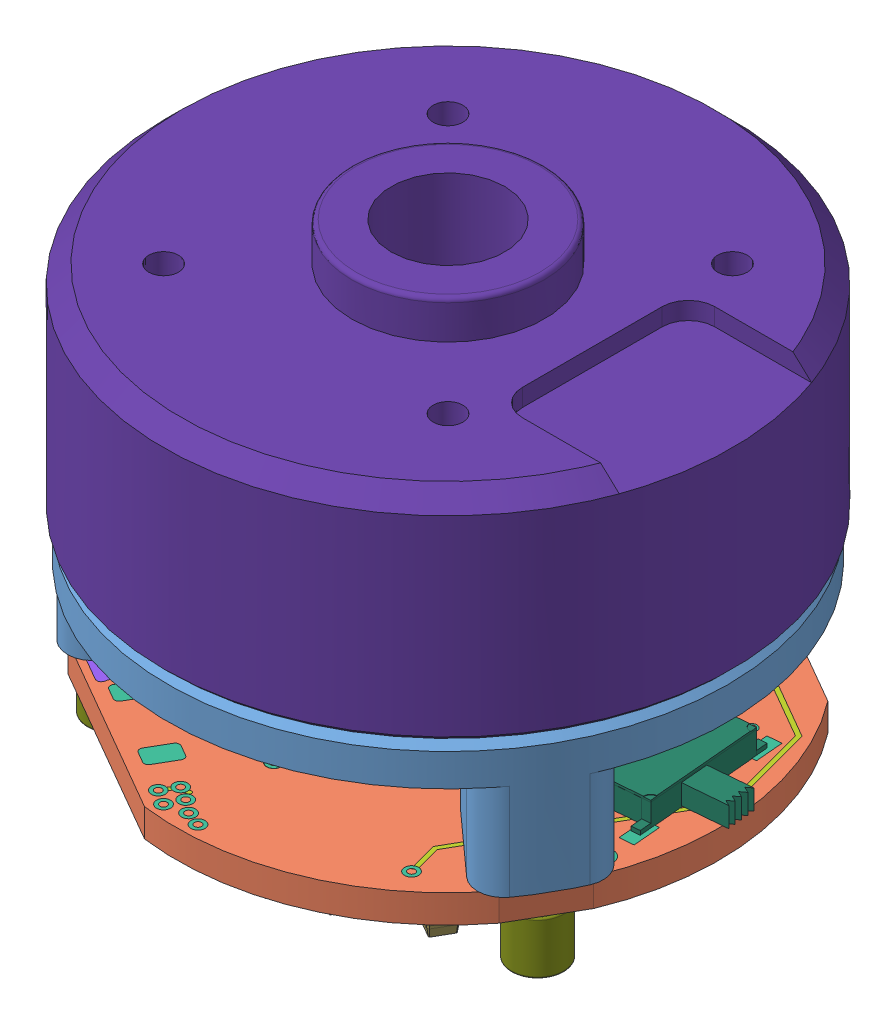
SolidWorks assembly 2804-特价电机, configuration 默认. Lengths in mm.
Overall size (40.92 27 40.14).
94 component instances, 53 part files, 8 mates.
Components (placement in the parent):
- 复件 零件1^2804-特价电机-1: 复件 零件1^2804-特价电机 [默认] x (0 0 -1) z (1 0 0) size (32 8.17 30.88) (virtual)
- S28P12-1: S28P12 [默认] at (0.0001 -9.6 0.0003) x (0.5 0 -0.866025) z (0 -1 0) size (28.6 30.74 6.15)
  - S28P12.step-1: S28P12.step [默认] at origin size (28.6 30.74 6.15)
    - Board_Geoms_db26.step-1: Board_Geoms_db26.step [默认] at origin size (28.6 30.74 1.88)
      - Pcb_db26.step-1: Pcb_db26.step [默认] at (-99.9998 99.9998 0) size (28.6 30.74 1.6)
      - topPads_db26.step-1: topPads_db26.step [默认] at (-99.9998 99.9998 0.02) size (27.56 29.1 0.01)
      - topTracks_db26.step-1: topTracks_db26.step [默认] at (-99.9998 99.9998 0.01) size (26.54 27.25 0.49)
      - topZones_db26.step-1: topZones_db26.step [默认] at (-99.9998 99.9998 0.01) size (16.88 29.66 0.02)
      - botPads_db26.step-1: botPads_db26.step [默认] at (-99.9998 99.9998 -1.62) size (27.7 29.1 0.01)
      - botTracks_db26.step-1: botTracks_db26.step [默认] at (-99.9998 99.9998 -1.61) size (26.06 27.6 0.02)
      - botZones_db26.step-1: botZones_db26.step [默认] at (-99.9998 99.9998 -1.61) size (24.07 13.81 0.01)
    - Step_Models_db26.step-1: Step_Models_db26.step [默认] at origin size (26.96 28.57 6.15)
      - Top_db26.step-1: Top_db26.step [默认] at origin size (24.86 27.45 1.59)
        - U4_PWP059_00006012a0b9.step-1: U4_PWP059_00006012a0b9.step [默认] at (-0.0198 -8.0402 0) x (0 1 0) z (1 0 0) size (6.4 1.2 9.7)
          - PWP28.step-1: PWP28.step [默认] at origin size (1 0.75 0.24)
          - PWP029.step-1: PWP029.step [默认] at origin size (1 0.75 0.24)
          - PWP030.step-1: PWP030.step [默认] at origin size (1 0.75 0.24)
          - PWP031.step-1: PWP031.step [默认] at origin size (1 0.75 0.24)
          - PWP032.step-1: PWP032.step [默认] at origin size (1 0.75 0.24)
          - PWP033.step-1: PWP033.step [默认] at origin size (1 0.75 0.24)
          - PWP034.step-1: PWP034.step [默认] at origin size (1 0.75 0.24)
          - PWP035.step-1: PWP035.step [默认] at origin size (1 0.75 0.24)
          - PWP036.step-1: PWP036.step [默认] at origin size (1 0.75 0.24)
          - PWP037.step-1: PWP037.step [默认] at origin size (1 0.75 0.24)
          - PWP038.step-1: PWP038.step [默认] at origin size (1 0.75 0.24)
          - PWP039.step-1: PWP039.step [默认] at origin size (1 0.75 0.24)
          - PWP040.step-1: PWP040.step [默认] at origin size (1 0.75 0.24)
          - PWP041.step-1: PWP041.step [默认] at origin size (1 0.75 0.24)
          - PWP042.step-1: PWP042.step [默认] at origin size (1 0.75 0.24)
          - PWP043.step-1: PWP043.step [默认] at origin size (1 0.75 0.24)
          - PWP044.step-1: PWP044.step [默认] at origin size (1 0.75 0.24)
          - PWP045.step-1: PWP045.step [默认] at origin size (1 0.75 0.24)
          - PWP046.step-1: PWP046.step [默认] at origin size (1 0.75 0.24)
          - PWP047.step-1: PWP047.step [默认] at origin size (1 0.75 0.24)
          - PWP048.step-1: PWP048.step [默认] at origin size (1 0.75 0.24)
          - PWP049.step-1: PWP049.step [默认] at origin size (1 0.75 0.24)
          - PWP050.step-1: PWP050.step [默认] at origin size (1 0.75 0.24)
          - PWP051.step-1: PWP051.step [默认] at origin size (1 0.75 0.24)
          - PWP052.step-1: PWP052.step [默认] at origin size (1 0.75 0.24)
          - PWP053.step-1: PWP053.step [默认] at origin size (1 0.75 0.24)
          - PWP054.step-1: PWP054.step [默认] at origin size (1 0.75 0.24)
          - PWP055.step-1: PWP055.step [默认] at origin size (1 0.75 0.24)
          - PWP056.step-1: PWP056.step [默认] at origin size (0.55 0.05 0.55)
          - PWP057.step-1: PWP057.step [默认] at origin size (4.4 1.06 9.7)
          - PWP058.step-1: PWP058.step [默认] at origin size (2.75 0.25 5.23)
        - C2_C_0603_1608Metric_00006005682b.step-1: C2_C_0603_1608Metric_00006005682b.step [默认] at (-4.7929 -0.2178 0) x (0 1 0) z (0 0 1) size (1.6 0.8 0.8)
        - C2_C_0603_1608Metric_00006005682b.step-2: C2_C_0603_1608Metric_00006005682b.step [默认] at (-6.2929 -0.2378 0) x (0 1 0) z (0 0 1) size (1.6 0.8 0.8)
        - C2_C_0603_1608Metric_00006005682b.step-3: C2_C_0603_1608Metric_00006005682b.step [默认] at (-5.9698 -10.4127 0) x (0 -1 0) z (0 0 1) size (1.6 0.8 0.8)
        - C2_C_0603_1608Metric_00006005682b.step-4: C2_C_0603_1608Metric_00006005682b.step [默认] at (-9.9829 6.3622 0) x (0 1 0) z (0 0 1) size (1.6 0.8 0.8)
        - C2_C_0603_1608Metric_00006005682b.step-5: C2_C_0603_1608Metric_00006005682b.step [默认] at (7.5102 -10.7002 0) x (0 1 0) z (0 0 1) size (1.6 0.8 0.8)
        - C2_C_0603_1608Metric_00006005682b.step-6: C2_C_0603_1608Metric_00006005682b.step [默认] at (-2.0229 9.3422 0) x (0 1 0) z (0 0 1) size (1.6 0.8 0.8)
        - C2_C_0603_1608Metric_00006005682b.step-7: C2_C_0603_1608Metric_00006005682b.step [默认] at (-5.2298 -13.0102 0) size (1.6 0.8 0.8)
        - C2_C_0603_1608Metric_00006005682b.step-8: C2_C_0603_1608Metric_00006005682b.step [默认] at (-7.4598 -10.4002 0) x (0 1 0) z (0 0 1) size (1.6 0.8 0.8)
        - C2_C_0603_1608Metric_00006005682b.step-9: C2_C_0603_1608Metric_00006005682b.step [默认] at (7.5302 -7.6827 0) x (0 -1 0) z (0 0 1) size (1.6 0.8 0.8)
        - D2_LED_0603_1608Metric_0000600568f0.step-1: D2_LED_0603_1608Metric_0000600568f0.step [默认] at (9.0171 -7.6853 0) x (0 1 0) z (0 0 1) size (1.6 0.8 1.1)
        - R1_R_0603_1608Metric_00006005698f.step-1: R1_R_0603_1608Metric_00006005698f.step [默认] at (10.6096 8.0922 0) x (-1 0 0) z (0 0 1) size (1.6 0.8 0.45)
        - R1_R_0603_1608Metric_00006005698f.step-2: R1_R_0603_1608Metric_00006005698f.step [默认] at (9.2771 -4.0278 0) x (0 1 0) z (0 0 1) size (1.6 0.8 0.45)
        - R1_R_0603_1608Metric_00006005698f.step-3: R1_R_0603_1608Metric_00006005698f.step [默认] at (-3.3129 -1.3653 0) x (0 -1 0) z (0 0 1) size (1.6 0.8 0.45)
        - R1_R_0603_1608Metric_00006005698f.step-4: R1_R_0603_1608Metric_00006005698f.step [默认] at (0.9171 9.3297 0) x (0 1 0) z (0 0 1) size (1.6 0.8 0.45)
        - R1_R_0603_1608Metric_00006005698f.step-5: R1_R_0603_1608Metric_00006005698f.step [默认] at (-1.8229 -1.3653 0) x (0 -1 0) z (0 0 1) size (1.6 0.8 0.45)
        - R1_R_0603_1608Metric_00006005698f.step-6: R1_R_0603_1608Metric_00006005698f.step [默认] at (6.0402 -7.6827 0) x (0 -1 0) z (0 0 1) size (1.6 0.8 0.45)
        - SW1_SW_SPST_B3U-1000P_000060056a0b.step-1: SW1_SW_SPST_B3U-1000P_000060056a0b.step [默认] at (4.6571 9.5022 0) size (4 2.51 1.59)
        - U3_SOT_89_3_000060056a8b.step-1: U3_SOT_89_3_000060056a8b.step [默认] at (-6.7429 8.2822 0) x (0 -1 0) z (0 0 1) size (4 4.5 1.52)
        - C2_C_0603_1608Metric_00006005682b.step-10: C2_C_0603_1608Metric_00006005682b.step [默认] at (10.6096 6.6222 0) x (-1 0 0) z (0 0 1) size (1.6 0.8 0.8)
        - D1_D_0603_00006081285b.step-1: D1_D_0603_00006081285b.step [默认] at (11.3571 1.4022 0) x (0 -1 0) z (0 0 1) size (1.6 0.87 0.66)
        - C2_C_0603_1608Metric_00006005682b.step-11: C2_C_0603_1608Metric_00006005682b.step [默认] at (-6.2729 4.2322 0) x (0 1 0) z (0 0 1) size (1.6 0.8 0.8)
        - C2_C_0603_1608Metric_00006005682b.step-12: C2_C_0603_1608Metric_00006005682b.step [默认] at (7.7671 -4.0153 0) x (0 1 0) z (0 0 1) size (1.6 0.8 0.8)
        - C2_C_0603_1608Metric_00006005682b.step-13: C2_C_0603_1608Metric_00006005682b.step [默认] at (-5.5329 1.9922 0) size (1.6 0.8 0.8)
        - C2_C_0603_1608Metric_00006005682b.step-14: C2_C_0603_1608Metric_00006005682b.step [默认] at (-0.5529 9.3297 0) x (0 -1 0) z (0 0 1) size (1.6 0.8 0.8)
        - C2_C_0603_1608Metric_00006005682b.step-15: C2_C_0603_1608Metric_00006005682b.step [默认] at (11.3571 4.3947 0) x (0 1 0) z (0 0 1) size (1.6 0.8 0.8)
        - C2_C_0603_1608Metric_00006005682b.step-16: C2_C_0603_1608Metric_00006005682b.step [默认] at (-2.5729 0.8622 0) size (1.6 0.8 0.8)
        - R1_R_0603_1608Metric_00006005698f.step-7: R1_R_0603_1608Metric_00006005698f.step [默认] at (-4.8029 4.2097 0) x (0 -1 0) z (0 0 1) size (1.6 0.8 0.45)
        - R1_R_0603_1608Metric_00006005698f.step-8: R1_R_0603_1608Metric_00006005698f.step [默认] at (-5.5529 -2.4578 0) size (1.6 0.8 0.45)
        - U5_LQFP_48_7x7mm_P05mm_000060d40c5b.step-1: U5_LQFP_48_7x7mm_P05mm_000060d40c5b.step [默认] at (5.1427 2.698 0) size (9 9 1.5)
        - R1_R_0603_1608Metric_00006005698f.step-9: R1_R_0603_1608Metric_00006005698f.step [默认] at (6.1396 11.9422 0) x (-1 0 0) z (0 0 1) size (1.6 0.8 0.45)
        - R1_R_0603_1608Metric_00006005698f.step-10: R1_R_0603_1608Metric_00006005698f.step [默认] at (6.1971 -4.0378 0) x (0 1 0) z (0 0 1) size (1.6 0.8 0.45)
        - C2_C_0603_1608Metric_00006005682b.step-17: C2_C_0603_1608Metric_00006005682b.step [默认] at (-9.9829 9.3522 0) x (0 1 0) z (0 0 1) size (1.6 0.8 0.8)
        - C2_C_0603_1608Metric_00006005682b.step-18: C2_C_0603_1608Metric_00006005682b.step [默认] at (-3.4929 9.3497 0) x (0 -1 0) z (0 0 1) size (1.6 0.8 0.8)
        - C2_C_0603_1608Metric_00006005682b.step-19: C2_C_0603_1608Metric_00006005682b.step [默认] at (-7.3579 11.5722 0) size (1.6 0.8 0.8)
        - C22_C_0805_2012Metric_82ecb5eb1270.step-1: C22_C_0805_2012Metric_82ecb5eb1270.step [默认] at (-12.0729 3.8822 0) x (-1 0 0) z (0 0 1) size (2 1.25 1.25)
        - C22_C_0805_2012Metric_82ecb5eb1270.step-2: C22_C_0805_2012Metric_82ecb5eb1270.step [默认] at (-12.0729 1.9122 0) x (-1 0 0) z (0 0 1) size (2 1.25 1.25)
        - C22_C_0805_2012Metric_82ecb5eb1270.step-3: C22_C_0805_2012Metric_82ecb5eb1270.step [默认] at (-12.0629 -4.0078 0) x (-1 0 0) z (0 0 1) size (2 1.25 1.25)
        - C22_C_0805_2012Metric_82ecb5eb1270.step-4: C22_C_0805_2012Metric_82ecb5eb1270.step [默认] at (-12.0729 -0.0578 0) x (-1 0 0) z (0 0 1) size (2 1.25 1.25)
        - VR1_SOT_23_081ca162a7f8.step-1: VR1_SOT_23_081ca162a7f8.step [默认] at (-3.9429 12.5422 0) x (-1 0 0) z (0 0 1) size (2.5 3 1.2)
        - C2_C_0603_1608Metric_00006005682b.step-20: C2_C_0603_1608Metric_00006005682b.step [默认] at (3.1571 11.9522 0) x (-1 0 0) z (0 0 1) size (1.6 0.8 0.8)
        - C22_C_0805_2012Metric_82ecb5eb1270.step-5: C22_C_0805_2012Metric_82ecb5eb1270.step [默认] at (-12.0629 -2.0378 0) x (-1 0 0) z (0 0 1) size (2 1.25 1.25)
      - Bot_db26.step-1: Bot_db26.step [默认] at origin size (16.88 18.18 3.54)
        - J4_SM04B-SRSS_000060d40966[2].step-1: J4_SM04B-SRSS_000060d40966[2].step [默认] at (9.988 -0.0178 -1.3) x (0 -1 0) z (1 0 0) size (6 2.96 4.95)
        - U2_SOIC_8_39x49mm_P127mm_000060d5d58d.step-1: U2_SOIC_8_39x49mm_P127mm_000060d5d58d.step [默认] at (0.0002 -0.0002 -1.6) x (1 0 0) z (0 0 -1) size (6 4.9 1.75)
        - SW2_Selector Switch - MSK1103_000061156a95.step-1: SW2_Selector Switch - MSK1103_000061156a95.step [默认] at (2.8725 14.2724 -1.6) x (0.819152 -0.573576 0) z (0.573576 0.819152 0) size (7.98 2.01 6.19)
- 复件 零件19^2804-特价电机-1: 复件 零件19^2804-特价电机 [默认] at (-12.1244 -12.6 7) x (0.999963 0 0.008553) z (-0.008553 0 0.999963) size (3 3 3) (virtual)
- 复件 零件75^2804-特价电机-1: 复件 零件75^2804-特价电机 [默认] at origin size (32.5 20 32.5) (virtual)
- 复件 零件19^2804-特价电机-2: 复件 零件19^2804-特价电机 [默认] at (0 -12.6 -14) x (-0.507389 0 0.861717) z (-0.861717 0 -0.507389) size (3 3 3) (virtual)
- 复件 零件19^2804-特价电机-3: 复件 零件19^2804-特价电机 [默认] at (12.1244 -12.6 7) x (-0.492575 0 -0.87027) z (0.87027 0 -0.492575) size (3 3 3) (virtual)
Mates (geometry in assembly coordinates):
- 重合1: coincident anti-aligned: plane of 复件 零件75^装配体1_2805特价电机-2轴-1 through (0 0 0) normal (0 -1 0); plane of 复件 零件1^装配体1_2805特价电机-2轴-1 through (0 0 0) normal (0 1 0)
- 同心1: concentric aligned: cylinder of 复件 零件75^装配体1_2805特价电机-2轴-1 through (11.5 5 0) axis (0 -1 0) radius 0.85; cylinder of 复件 零件1^装配体1_2805特价电机-2轴-1 through (11.5 0 0) axis (0 -1 0) radius 1.1
- 同心2: concentric anti-aligned: cylinder of 复件 零件75^装配体1_2805特价电机-2轴-1 through (0 12.2 0) axis (0 -1 0) radius 16.25; cylinder of 复件 零件1^装配体1_2805特价电机-2轴-1 through (0 -8 0) axis (0 1 0) radius 16
- 重合2: coincident anti-aligned: plane of 复件 零件1^装配体1_2805特价电机-2轴-1 through (0 -8 0) normal (0 -1 0); plane of S28P12-1/S28P12.step-1/Board_Geoms_db26.step-1/Pcb_db26.step-1 through (0.0001 -8 0.0002) normal (0 1 0)
- 同心4: concentric anti-aligned: cylinder of 复件 零件1^装配体1_2805特价电机-2轴-1 through (0 -8 -14) axis (0 1 0) radius 0.925; cylinder of S28P12-1/S28P12.step-1/Board_Geoms_db26.step-1/Pcb_db26.step-1 through (0 -9.6 -14) axis (0 -1 0) radius 1.1
- 同心3: concentric aligned: cylinder of 复件 零件75^装配体1_2805特价电机-2轴-1 through (0 12.2 0) axis (0 -1 0) radius 16.25; cylinder of S28P12-1/S28P12.step-1/Board_Geoms_db26.step-1/Pcb_db26.step-1 through (0 -9.6 0) axis (0 -1 0) radius 15.4963
- 重合3: coincident anti-aligned: plane of S28P12-1/S28P12.step-1/Board_Geoms_db26.step-1/Pcb_db26.step-1 through (0.0001 -9.6 0.0002) normal (0 -1 0); plane of 复件 零件19^装配体1_2805特价电机-2轴-1 through (-12.1244 -9.6 7) normal (0 1 0)
- 同心5: concentric aligned: cylinder of S28P12-1/S28P12.step-1/Board_Geoms_db26.step-1/Pcb_db26.step-1 through (-12.1244 -9.6 7) axis (0 -1 0) radius 1.1; cylinder of 复件 零件19^装配体1_2805特价电机-2轴-1 through (-12.1244 -9.6 7) axis (0 -1 0) radius 1.5
